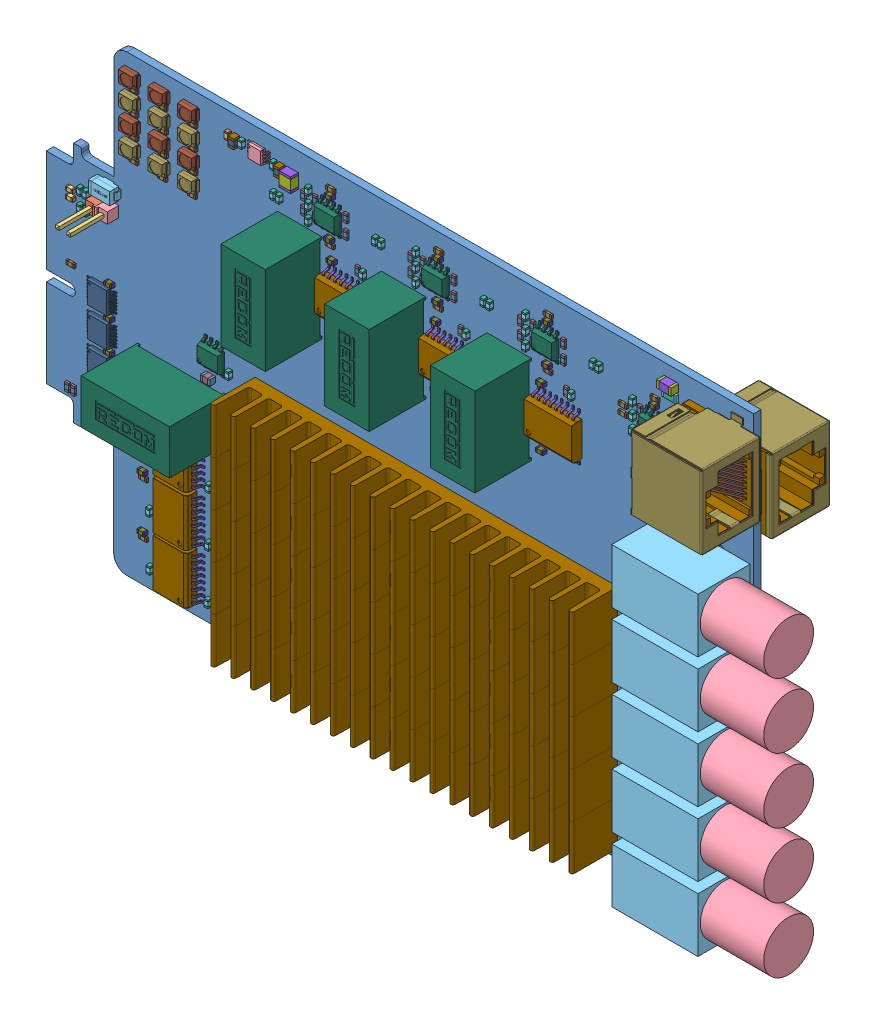
SolidWorks assembly 1166V10, configuration Standard. Lengths in mm. (continued)
Components (placement in the parent): (continued)
- 1166V10.step-1: 1166V10.step [Standard] at origin size (170.01 100 28.53) (continued)
  - C233.step-1: C233.step [Standard] at origin size (0.82 1.6 0.9) (continued)
    - 6549602528.step-1: 6549602528.step [Standard] at (39.6 30.325 -2.522) size (0.82 0.35 0.9) (continued)
      - Extruded-0.step-1: Extruded-0.step [Standard] at origin size (0.82 0.35 0.9)
    - 6549602528.step-2: 6549602528.step [Standard] at (39.6 31.575 -2.522) size (0.82 0.35 0.9)
      - Extruded-0.step-1: Extruded-0.step [Standard] at origin size (0.82 0.35 0.9)
    - 6547668352.step-1: 6547668352.step [Standard] at (39.6 30.95 -2.522) size (0.82 0.9 0.9)
      - Extruded.step-1: Extruded.step [Standard] at origin size (0.82 0.9 0.9)
  - C232.step-1: C232.step [Standard] at origin size (0.82 1.6 0.9)
    - 6547668352.step-1: 6547668352.step [Standard] at (106.1 91.15 0) size (0.82 0.9 0.9)
      - Extruded.step-1: Extruded.step [Standard] at origin size (0.82 0.9 0.9)
    - 6549602528.step-1: 6549602528.step [Standard] at (106.1 91.775 0) size (0.82 0.35 0.9)
      - Extruded-0.step-1: Extruded-0.step [Standard] at origin size (0.82 0.35 0.9)
    - 6549602528.step-2: 6549602528.step [Standard] at (106.1 90.525 0) size (0.82 0.35 0.9)
      - Extruded-0.step-1: Extruded-0.step [Standard] at origin size (0.82 0.35 0.9)
  - C231.step-1: C231.step [Standard] at origin size (0.82 1.6 0.9)
    - 6547668352.step-1: 6547668352.step [Standard] at (106.1 94.05 0) size (0.82 0.9 0.9)
      - Extruded.step-1: Extruded.step [Standard] at origin size (0.82 0.9 0.9)
    - 6549602528.step-1: 6549602528.step [Standard] at (106.1 94.675 0) size (0.82 0.35 0.9)
      - Extruded-0.step-1: Extruded-0.step [Standard] at origin size (0.82 0.35 0.9)
    - 6549602528.step-2: 6549602528.step [Standard] at (106.1 93.425 0) size (0.82 0.35 0.9)
      - Extruded-0.step-1: Extruded-0.step [Standard] at origin size (0.82 0.35 0.9)
  - R101.step-1: R101.step [Standard] at origin size (1.85 0.85 0.45)
    - 6547171712.step-1: 6547171712.step [Standard] at (4.95 53.6 0) size (0.45 0.85 0.45)
      - Extruded-5.step-1: Extruded-5.step [Standard] at origin size (0.45 0.85 0.45)
    - 6547171712.step-2: 6547171712.step [Standard] at (6.35 53.6 0) size (0.45 0.85 0.45)
      - Extruded-5.step-1: Extruded-5.step [Standard] at origin size (0.45 0.85 0.45)
    - 6547171152.step-1: 6547171152.step [Standard] at (5.65 53.6 0) size (0.95 0.85 0.45)
      - Extruded-6.step-1: Extruded-6.step [Standard] at origin size (0.95 0.85 0.45)
  - CF101.step-1: CF101.step [Standard] at origin size (1.6 0.82 0.9)
    - 6547664912.step-1: 6547664912.step [Standard] at (13.725 54.2 0) size (0.35 0.82 0.9)
      - Extruded-10.step-1: Extruded-10.step [Standard] at origin size (0.35 0.82 0.9)
    - 6547664912.step-2: 6547664912.step [Standard] at (14.975 54.2 0) size (0.35 0.82 0.9)
      - Extruded-10.step-1: Extruded-10.step [Standard] at origin size (0.35 0.82 0.9)
    - 6547664352.step-1: 6547664352.step [Standard] at (14.35 54.2 0) size (0.9 0.82 0.9)
      - Extruded-9.step-1: Extruded-9.step [Standard] at origin size (0.9 0.82 0.9)
  - PS202.step-1: PS202.step [Standard] at origin size (19.5 9.8 16.6)
    - RxxPxx_X2_R.step-1: RxxPxx_X2_R.step [Standard] at (29.9099 40.6999 0.51) x (1 0 0) z (0 -1 0) size (0.5 4.6 0.25)
    - RxxPxx_X2_R-24.step-1: RxxPxx_X2_R-24.step [Standard] at (29.9099 40.6999 0.51) x (1 0 0) z (0 -1 0) size (0.5 4.6 0.25)
    - RxxPxx_X2_R-25.step-1: RxxPxx_X2_R-25.step [Standard] at (29.9099 40.6999 0.51) x (1 0 0) z (0 -1 0) size (19.5 12.5 9.8)
    - RxxPxx_X2_R-26.step-1: RxxPxx_X2_R-26.step [Standard] at (29.9099 40.6999 0.51) x (1 0 0) z (0 -1 0) size (18.5 11.5 8.9)
    - RxxPxx_X2_R-27.step-1: RxxPxx_X2_R-27.step [Standard] at (29.9099 40.6999 0.51) x (1 0 0) z (0 -1 0) size (0.5 4.6 0.25)
    - RxxPxx_X2_R-28.step-1: RxxPxx_X2_R-28.step [Standard] at (29.9099 40.6999 0.51) x (1 0 0) z (0 -1 0) size (0.5 4.6 0.25)
  - PS401.step-1: PS401.step [Standard] at origin size (9.8 19.5 16.6)
    - RxxPxx_X2_R.step-1: RxxPxx_X2_R.step [Standard] at (55.8999 76.45 0.51) x (0 -1 0) z (-1 0 0) size (0.5 4.6 0.25)
    - RxxPxx_X2_R-24.step-1: RxxPxx_X2_R-24.step [Standard] at (55.8999 76.45 0.51) x (0 -1 0) z (-1 0 0) size (0.5 4.6 0.25)
    - RxxPxx_X2_R-25.step-1: RxxPxx_X2_R-25.step [Standard] at (55.8999 76.45 0.51) x (0 -1 0) z (-1 0 0) size (19.5 12.5 9.8)
    - RxxPxx_X2_R-26.step-1: RxxPxx_X2_R-26.step [Standard] at (55.8999 76.45 0.51) x (0 -1 0) z (-1 0 0) size (18.5 11.5 8.9)
    - RxxPxx_X2_R-27.step-1: RxxPxx_X2_R-27.step [Standard] at (55.8999 76.45 0.51) x (0 -1 0) z (-1 0 0) size (0.5 4.6 0.25)
    - RxxPxx_X2_R-28.step-1: RxxPxx_X2_R-28.step [Standard] at (55.8999 76.45 0.51) x (0 -1 0) z (-1 0 0) size (0.5 4.6 0.25)
  - PS301.step-1: PS301.step [Standard] at origin size (9.8 19.5 16.6)
    - RxxPxx_X2_R.step-1: RxxPxx_X2_R.step [Standard] at (78.7999 76.45 0.51) x (0 -1 0) z (-1 0 0) size (0.5 4.6 0.25)
    - RxxPxx_X2_R-24.step-1: RxxPxx_X2_R-24.step [Standard] at (78.7999 76.45 0.51) x (0 -1 0) z (-1 0 0) size (0.5 4.6 0.25)
    - RxxPxx_X2_R-25.step-1: RxxPxx_X2_R-25.step [Standard] at (78.7999 76.45 0.51) x (0 -1 0) z (-1 0 0) size (19.5 12.5 9.8)
    - RxxPxx_X2_R-26.step-1: RxxPxx_X2_R-26.step [Standard] at (78.7999 76.45 0.51) x (0 -1 0) z (-1 0 0) size (18.5 11.5 8.9)
    - RxxPxx_X2_R-27.step-1: RxxPxx_X2_R-27.step [Standard] at (78.7999 76.45 0.51) x (0 -1 0) z (-1 0 0) size (0.5 4.6 0.25)
    - RxxPxx_X2_R-28.step-1: RxxPxx_X2_R-28.step [Standard] at (78.7999 76.45 0.51) x (0 -1 0) z (-1 0 0) size (0.5 4.6 0.25)
  - L402.step-1: L402.step [Standard] at origin size (1.8 2 1.8)
    - 6547443440.step-1: 6547443440.step [Standard] at (56.3 66.0999 -3.422) size (1.8 0.5 1.8)
      - Extruded-29.step-1: Extruded-29.step [Standard] at origin size (1.8 0.5 1.8)
    - 6547443440.step-2: 6547443440.step [Standard] at (56.3 64.6 -3.422) size (1.8 0.5 1.8)
      - Extruded-29.step-1: Extruded-29.step [Standard] at origin size (1.8 0.5 1.8)
    - 6547443040.step-1: 6547443040.step [Standard] at (56.3 65.3499 -3.422) size (1.8 1 1.8)
      - Extruded-30.step-1: Extruded-30.step [Standard] at origin size (1.8 1 1.8)
  - L401.step-1: L401.step [Standard] at origin size (1.8 2 1.8)
    - 6547443440.step-1: 6547443440.step [Standard] at (56.9 89.3999 -3.422) size (1.8 0.5 1.8)
      - Extruded-29.step-1: Extruded-29.step [Standard] at origin size (1.8 0.5 1.8)
    - 6547443440.step-2: 6547443440.step [Standard] at (56.9 87.9 -3.422) size (1.8 0.5 1.8)
      - Extruded-29.step-1: Extruded-29.step [Standard] at origin size (1.8 0.5 1.8)
    - 6547443040.step-1: 6547443040.step [Standard] at (56.8999 88.6499 -3.422) size (1.8 1 1.8)
      - Extruded-30.step-1: Extruded-30.step [Standard] at origin size (1.8 1 1.8)
  - L302.step-1: L302.step [Standard] at origin size (1.8 2 1.8)
    - 6547443440.step-1: 6547443440.step [Standard] at (79.2 66.0999 -3.422) size (1.8 0.5 1.8)
      - Extruded-29.step-1: Extruded-29.step [Standard] at origin size (1.8 0.5 1.8)
    - 6547443440.step-2: 6547443440.step [Standard] at (79.2 64.6 -3.422) size (1.8 0.5 1.8)
      - Extruded-29.step-1: Extruded-29.step [Standard] at origin size (1.8 0.5 1.8)
    - 6547443040.step-1: 6547443040.step [Standard] at (79.1999 65.3499 -3.422) size (1.8 1 1.8)
      - Extruded-30.step-1: Extruded-30.step [Standard] at origin size (1.8 1 1.8)
  - L301.step-1: L301.step [Standard] at origin size (1.8 2 1.8)
    - 6547443440.step-1: 6547443440.step [Standard] at (79.4 89.3999 -3.422) size (1.8 0.5 1.8)
      - Extruded-29.step-1: Extruded-29.step [Standard] at origin size (1.8 0.5 1.8)
    - 6547443440.step-2: 6547443440.step [Standard] at (79.4 87.9 -3.422) size (1.8 0.5 1.8)
      - Extruded-29.step-1: Extruded-29.step [Standard] at origin size (1.8 0.5 1.8)
    - 6547443040.step-1: 6547443040.step [Standard] at (79.3999 88.6499 -3.422) size (1.8 1 1.8)
      - Extruded-30.step-1: Extruded-30.step [Standard] at origin size (1.8 1 1.8)
  - J401.step-1: J401.step [Standard] at origin size (33 12 11.5)
    - 6544611248.step-1: 6544611248.step [Standard] at (146.5 8.5 0.8) size (19 12 11.5)
      - Extruded-21.step-1: Extruded-21.step [Standard] at origin size (19 12 11.5)
    - 6544611488.step-1: 6544611488.step [Standard] at (170 8.5434 6.3) x (0 -1 0) z (-1 0 0) size (11 11 14)
      - Cylinder.step-1: Cylinder.step [Standard] at origin size (11 11 14)
  - J301.step-1: J301.step [Standard] at origin size (33 12 11.5)
    - 6544611248.step-1: 6544611248.step [Standard] at (146.5 22.8 0.8) size (19 12 11.5)
      - Extruded-21.step-1: Extruded-21.step [Standard] at origin size (19 12 11.5)
    - 6544611488.step-1: 6544611488.step [Standard] at (170 22.8434 6.3) x (0 -1 0) z (-1 0 0) size (11 11 14)
      - Cylinder.step-1: Cylinder.step [Standard] at origin size (11 11 14)
  - CF405.step-1: CF405.step [Standard] at origin size (0.82 1.6 0.9)
    - 6547668352.step-1: 6547668352.step [Standard] at (23.2 26.35 0) size (0.82 0.9 0.9)
      - Extruded.step-1: Extruded.step [Standard] at origin size (0.82 0.9 0.9)
    - 6549602528.step-1: 6549602528.step [Standard] at (23.2 26.975 0) size (0.82 0.35 0.9)
      - Extruded-0.step-1: Extruded-0.step [Standard] at origin size (0.82 0.35 0.9)
    - 6549602528.step-2: 6549602528.step [Standard] at (23.2 25.725 0) size (0.82 0.35 0.9)
      - Extruded-0.step-1: Extruded-0.step [Standard] at origin size (0.82 0.35 0.9)
  - CF402.step-1: CF402.step [Standard] at origin size (2.1 1.25 1.3)
    - 6545928368.step-1: 6545928368.step [Standard] at (58.7 64.6 -2.922) size (0.5 1.25 1.3)
      - Extruded-16.step-1: Extruded-16.step [Standard] at origin size (0.5 1.25 1.3)
    - 6545928368.step-2: 6545928368.step [Standard] at (60.3 64.6 -2.922) size (0.5 1.25 1.3)
      - Extruded-16.step-1: Extruded-16.step [Standard] at origin size (0.5 1.25 1.3)
    - 6545927808.step-1: 6545927808.step [Standard] at (59.5 64.6 -2.922) size (1.1 1.25 1.3)
      - Extruded-15.step-1: Extruded-15.step [Standard] at origin size (1.1 1.25 1.3)
  - CF401.step-1: CF401.step [Standard] at origin size (2.1 1.25 1.3)
    - 6545928368.step-1: 6545928368.step [Standard] at (58.7 66.4 -2.922) size (0.5 1.25 1.3)
      - Extruded-16.step-1: Extruded-16.step [Standard] at origin size (0.5 1.25 1.3)
    - 6545928368.step-2: 6545928368.step [Standard] at (60.3 66.4 -2.922) size (0.5 1.25 1.3)
      - Extruded-16.step-1: Extruded-16.step [Standard] at origin size (0.5 1.25 1.3)
    - 6545927808.step-1: 6545927808.step [Standard] at (59.5 66.4 -2.922) size (1.1 1.25 1.3)
      - Extruded-15.step-1: Extruded-15.step [Standard] at origin size (1.1 1.25 1.3)
  - CF403.step-1: CF403.step [Standard] at origin size (1.6 0.82 0.9)
    - 6547664352.step-1: 6547664352.step [Standard] at (63.35 83.1 0) size (0.9 0.82 0.9)
      - Extruded-9.step-1: Extruded-9.step [Standard] at origin size (0.9 0.82 0.9)
    - 6547664912.step-1: 6547664912.step [Standard] at (63.975 83.1 0) size (0.35 0.82 0.9)
      - Extruded-10.step-1: Extruded-10.step [Standard] at origin size (0.35 0.82 0.9)
    - 6547664912.step-2: 6547664912.step [Standard] at (62.725 83.1 0) size (0.35 0.82 0.9)
      - Extruded-10.step-1: Extruded-10.step [Standard] at origin size (0.35 0.82 0.9)
  - CF305.step-1: CF305.step [Standard] at origin size (0.82 1.6 0.9)
    - 6547668352.step-1: 6547668352.step [Standard] at (23.2 15.25 0) size (0.82 0.9 0.9)
      - Extruded.step-1: Extruded.step [Standard] at origin size (0.82 0.9 0.9)
    - 6549602528.step-1: 6549602528.step [Standard] at (23.2 15.875 0) size (0.82 0.35 0.9)
      - Extruded-0.step-1: Extruded-0.step [Standard] at origin size (0.82 0.35 0.9)
    - 6549602528.step-2: 6549602528.step [Standard] at (23.2 14.625 0) size (0.82 0.35 0.9)
      - Extruded-0.step-1: Extruded-0.step [Standard] at origin size (0.82 0.35 0.9)
  - CF302.step-1: CF302.step [Standard] at origin size (2.1 1.25 1.3)
    - 6545928368.step-1: 6545928368.step [Standard] at (81.6 64.6 -2.922) size (0.5 1.25 1.3)
      - Extruded-16.step-1: Extruded-16.step [Standard] at origin size (0.5 1.25 1.3)
    - 6545928368.step-2: 6545928368.step [Standard] at (83.2 64.6 -2.922) size (0.5 1.25 1.3)
      - Extruded-16.step-1: Extruded-16.step [Standard] at origin size (0.5 1.25 1.3)
    - 6545927808.step-1: 6545927808.step [Standard] at (82.4 64.6 -2.922) size (1.1 1.25 1.3)
      - Extruded-15.step-1: Extruded-15.step [Standard] at origin size (1.1 1.25 1.3)
  - CF301.step-1: CF301.step [Standard] at origin size (2.1 1.25 1.3)
    - 6545928368.step-1: 6545928368.step [Standard] at (81.6 66.4 -2.922) size (0.5 1.25 1.3)
      - Extruded-16.step-1: Extruded-16.step [Standard] at origin size (0.5 1.25 1.3)
    - 6545928368.step-2: 6545928368.step [Standard] at (83.2 66.4 -2.922) size (0.5 1.25 1.3)
      - Extruded-16.step-1: Extruded-16.step [Standard] at origin size (0.5 1.25 1.3)
    - 6545927808.step-1: 6545927808.step [Standard] at (82.4 66.4 -2.922) size (1.1 1.25 1.3)
      - Extruded-15.step-1: Extruded-15.step [Standard] at origin size (1.1 1.25 1.3)
  - CF303.step-1: CF303.step [Standard] at origin size (1.6 0.82 0.9)
    - 6547664352.step-1: 6547664352.step [Standard] at (86.25 83 0) size (0.9 0.82 0.9)
      - Extruded-9.step-1: Extruded-9.step [Standard] at origin size (0.9 0.82 0.9)
    - 6547664912.step-1: 6547664912.step [Standard] at (86.875 83 0) size (0.35 0.82 0.9)
      - Extruded-10.step-1: Extruded-10.step [Standard] at origin size (0.35 0.82 0.9)
    - 6547664912.step-2: 6547664912.step [Standard] at (85.625 83 0) size (0.35 0.82 0.9)
      - Extruded-10.step-1: Extruded-10.step [Standard] at origin size (0.35 0.82 0.9)
  - C410.step-1: C410.step [Standard] at origin size (1.6 0.82 0.9)
    - 6547664912.step-1: 6547664912.step [Standard] at (58.625 63.1 -2.522) size (0.35 0.82 0.9)
      - Extruded-10.step-1: Extruded-10.step [Standard] at origin size (0.35 0.82 0.9)
    - 6547664912.step-2: 6547664912.step [Standard] at (59.875 63.1 -2.522) size (0.35 0.82 0.9)
      - Extruded-10.step-1: Extruded-10.step [Standard] at origin size (0.35 0.82 0.9)
    - 6547664352.step-1: 6547664352.step [Standard] at (59.25 63.1 -2.522) size (0.9 0.82 0.9)
      - Extruded-9.step-1: Extruded-9.step [Standard] at origin size (0.9 0.82 0.9)
  - C409.step-1: C409.step [Standard] at origin size (3.2 1.6 1.7)
    - 6547445040.step-1: 6547445040.step [Standard] at (60.55 87.7 -3.322) size (2.2 1.6 1.7)
      - Extruded-23.step-1: Extruded-23.step [Standard] at origin size (2.2 1.6 1.7)
    - 6547444720.step-1: 6547444720.step [Standard] at (59.2 87.7 -3.322) size (0.5 1.6 1.7)
      - Extruded-22.step-1: Extruded-22.step [Standard] at origin size (0.5 1.6 1.7)
    - 6547444720.step-2: 6547444720.step [Standard] at (61.9 87.7 -3.322) size (0.5 1.6 1.7)
      - Extruded-22.step-1: Extruded-22.step [Standard] at origin size (0.5 1.6 1.7)
  - C408.step-1: C408.step [Standard] at origin size (3.2 1.6 1.7)
    - 6547445040.step-1: 6547445040.step [Standard] at (60.55 89.8 -3.322) size (2.2 1.6 1.7)
      - Extruded-23.step-1: Extruded-23.step [Standard] at origin size (2.2 1.6 1.7)
    - 6547444720.step-1: 6547444720.step [Standard] at (59.2 89.8 -3.322) size (0.5 1.6 1.7)
      - Extruded-22.step-1: Extruded-22.step [Standard] at origin size (0.5 1.6 1.7)
    - 6547444720.step-2: 6547444720.step [Standard] at (61.9 89.8 -3.322) size (0.5 1.6 1.7)
      - Extruded-22.step-1: Extruded-22.step [Standard] at origin size (0.5 1.6 1.7)
  - C407.step-1: C407.step [Standard] at origin size (5.7 5 2.5)
    - 6545673168.step-1: 6545673168.step [Standard] at (66.25 49.3 -4.122) size (4.4 5 2.5)
      - Extruded-31.step-1: Extruded-31.step [Standard] at origin size (4.4 5 2.5)
    - 6545673728.step-1: 6545673728.step [Standard] at (68.775 49.3 -4.122) size (0.65 5 2.5)
      - Extruded-32.step-1: Extruded-32.step [Standard] at origin size (0.65 5 2.5)
    - 6545673728.step-2: 6545673728.step [Standard] at (63.725 49.3 -4.122) size (0.65 5 2.5)
      - Extruded-32.step-1: Extruded-32.step [Standard] at origin size (0.65 5 2.5)
  - C406.step-1: C406.step [Standard] at origin size (5.7 5 2.5)
    - 6545673728.step-1: 6545673728.step [Standard] at (56.375 43.2 -4.122) size (0.65 5 2.5)
      - Extruded-32.step-1: Extruded-32.step [Standard] at origin size (0.65 5 2.5)
    - 6545673728.step-2: 6545673728.step [Standard] at (51.325 43.2 -4.122) size (0.65 5 2.5)
      - Extruded-32.step-1: Extruded-32.step [Standard] at origin size (0.65 5 2.5)
    - 6545673168.step-1: 6545673168.step [Standard] at (53.85 43.2 -4.122) size (4.4 5 2.5)
      - Extruded-31.step-1: Extruded-31.step [Standard] at origin size (4.4 5 2.5)
  - C405.step-1: C405.step [Standard] at origin size (5.7 5 2.5)
    - 6545673728.step-1: 6545673728.step [Standard] at (56.375 49.3 -4.122) size (0.65 5 2.5)
      - Extruded-32.step-1: Extruded-32.step [Standard] at origin size (0.65 5 2.5)
    - 6545673728.step-2: 6545673728.step [Standard] at (51.325 49.3 -4.122) size (0.65 5 2.5)
      - Extruded-32.step-1: Extruded-32.step [Standard] at origin size (0.65 5 2.5)
    - 6545673168.step-1: 6545673168.step [Standard] at (53.85 49.3 -4.122) size (4.4 5 2.5)
      - Extruded-31.step-1: Extruded-31.step [Standard] at origin size (4.4 5 2.5)
  - C404.step-1: C404.step [Standard] at origin size (5.7 5 2.5)
    - 6545673728.step-1: 6545673728.step [Standard] at (63.725 43.2 -4.122) size (0.65 5 2.5)
      - Extruded-32.step-1: Extruded-32.step [Standard] at origin size (0.65 5 2.5)
    - 6545673728.step-2: 6545673728.step [Standard] at (68.775 43.2 -4.122) size (0.65 5 2.5)
      - Extruded-32.step-1: Extruded-32.step [Standard] at origin size (0.65 5 2.5)
    - 6545673168.step-1: 6545673168.step [Standard] at (66.25 43.2 -4.122) size (4.4 5 2.5)
      - Extruded-31.step-1: Extruded-31.step [Standard] at origin size (4.4 5 2.5)
  - C310.step-1: C310.step [Standard] at origin size (1.6 0.82 0.9)
    - 6547664912.step-1: 6547664912.step [Standard] at (82.025 63 -2.522) size (0.35 0.82 0.9)
      - Extruded-10.step-1: Extruded-10.step [Standard] at origin size (0.35 0.82 0.9)
    - 6547664912.step-2: 6547664912.step [Standard] at (83.275 63 -2.522) size (0.35 0.82 0.9)
      - Extruded-10.step-1: Extruded-10.step [Standard] at origin size (0.35 0.82 0.9)
    - 6547664352.step-1: 6547664352.step [Standard] at (82.65 63 -2.522) size (0.9 0.82 0.9)
      - Extruded-9.step-1: Extruded-9.step [Standard] at origin size (0.9 0.82 0.9)
  - C309.step-1: C309.step [Standard] at origin size (3.2 1.6 1.7)
    - 6547445040.step-1: 6547445040.step [Standard] at (83.05 87.6 -3.322) size (2.2 1.6 1.7)
      - Extruded-23.step-1: Extruded-23.step [Standard] at origin size (2.2 1.6 1.7)
    - 6547444720.step-1: 6547444720.step [Standard] at (81.7 87.6 -3.322) size (0.5 1.6 1.7)
      - Extruded-22.step-1: Extruded-22.step [Standard] at origin size (0.5 1.6 1.7)
    - 6547444720.step-2: 6547444720.step [Standard] at (84.4 87.6 -3.322) size (0.5 1.6 1.7)
      - Extruded-22.step-1: Extruded-22.step [Standard] at origin size (0.5 1.6 1.7)
  - C308.step-1: C308.step [Standard] at origin size (3.2 1.6 1.7)
    - 6547445040.step-1: 6547445040.step [Standard] at (83.05 89.7 -3.322) size (2.2 1.6 1.7)
      - Extruded-23.step-1: Extruded-23.step [Standard] at origin size (2.2 1.6 1.7)
    - 6547444720.step-1: 6547444720.step [Standard] at (81.7 89.7 -3.322) size (0.5 1.6 1.7)
      - Extruded-22.step-1: Extruded-22.step [Standard] at origin size (0.5 1.6 1.7)
    - 6547444720.step-2: 6547444720.step [Standard] at (84.4 89.7 -3.322) size (0.5 1.6 1.7)
      - Extruded-22.step-1: Extruded-22.step [Standard] at origin size (0.5 1.6 1.7)
  - C307.step-1: C307.step [Standard] at origin size (5.7 5 2.5)
    - 6545673168.step-1: 6545673168.step [Standard] at (93.15 49.3 -4.122) size (4.4 5 2.5)
      - Extruded-31.step-1: Extruded-31.step [Standard] at origin size (4.4 5 2.5)
    - 6545673728.step-1: 6545673728.step [Standard] at (95.675 49.3 -4.122) size (0.65 5 2.5)
      - Extruded-32.step-1: Extruded-32.step [Standard] at origin size (0.65 5 2.5)
    - 6545673728.step-2: 6545673728.step [Standard] at (90.625 49.3 -4.122) size (0.65 5 2.5)
      - Extruded-32.step-1: Extruded-32.step [Standard] at origin size (0.65 5 2.5)
  - C306.step-1: C306.step [Standard] at origin size (5.7 5 2.5)
    - 6545673728.step-1: 6545673728.step [Standard] at (83.375 49.3 -4.122) size (0.65 5 2.5)
      - Extruded-32.step-1: Extruded-32.step [Standard] at origin size (0.65 5 2.5)
    - 6545673728.step-2: 6545673728.step [Standard] at (78.325 49.3 -4.122) size (0.65 5 2.5)
      - Extruded-32.step-1: Extruded-32.step [Standard] at origin size (0.65 5 2.5)
    - 6545673168.step-1: 6545673168.step [Standard] at (80.85 49.3 -4.122) size (4.4 5 2.5)
      - Extruded-31.step-1: Extruded-31.step [Standard] at origin size (4.4 5 2.5)
  - C305.step-1: C305.step [Standard] at origin size (5.7 5 2.5)
    - 6545673728.step-1: 6545673728.step [Standard] at (83.375 43.2 -4.122) size (0.65 5 2.5)
      - Extruded-32.step-1: Extruded-32.step [Standard] at origin size (0.65 5 2.5)
    - 6545673728.step-2: 6545673728.step [Standard] at (78.325 43.2 -4.122) size (0.65 5 2.5)
      - Extruded-32.step-1: Extruded-32.step [Standard] at origin size (0.65 5 2.5)
    - 6545673168.step-1: 6545673168.step [Standard] at (80.85 43.2 -4.122) size (4.4 5 2.5)
      - Extruded-31.step-1: Extruded-31.step [Standard] at origin size (4.4 5 2.5)
  - C304.step-1: C304.step [Standard] at origin size (5.7 5 2.5)
    - 6545673728.step-1: 6545673728.step [Standard] at (90.625 43.2 -4.122) size (0.65 5 2.5)
      - Extruded-32.step-1: Extruded-32.step [Standard] at origin size (0.65 5 2.5)
    - 6545673728.step-2: 6545673728.step [Standard] at (95.675 43.2 -4.122) size (0.65 5 2.5)
      - Extruded-32.step-1: Extruded-32.step [Standard] at origin size (0.65 5 2.5)
    - 6545673168.step-1: 6545673168.step [Standard] at (93.15 43.2 -4.122) size (4.4 5 2.5)
      - Extruded-31.step-1: Extruded-31.step [Standard] at origin size (4.4 5 2.5)
  - L101.step-1: L101.step [Standard] at origin size (1.6 0.8 0.8)
    - WE-CBF_0603_CBF.step-1: WE-CBF_0603_CBF.step [Standard] at (5.7637 68.0001 0.4) x (0 1 0) z (0 0 1) size (0.8 1.6 0.8)
      - L_tende.step-1: L_tende.step [Standard] at (0 -0.5 0) size (0.8 0.3 0.8)
      - L_tende.step-2: L_tende.step [Standard] at (0 0.5 0) x (-1 0 0) z (0 0 1) size (0.8 0.3 0.8)
      - base.step-1: base.step [Standard] at origin size (0.8 1 0.8)
  - C102.step-1: C102.step [Standard] at origin size (0.82 1.6 0.9)
    - 6547668352.step-1: 6547668352.step [Standard] at (9.2 68.85 0) size (0.82 0.9 0.9)
      - Extruded.step-1: Extruded.step [Standard] at origin size (0.82 0.9 0.9)
    - 6549602528.step-1: 6549602528.step [Standard] at (9.2 68.225 0) size (0.82 0.35 0.9)
      - Extruded-0.step-1: Extruded-0.step [Standard] at origin size (0.82 0.35 0.9)
    - 6549602528.step-2: 6549602528.step [Standard] at (9.2 69.475 0) size (0.82 0.35 0.9)
      - Extruded-0.step-1: Extruded-0.step [Standard] at origin size (0.82 0.35 0.9)
  - C101.step-1: C101.step [Standard] at origin size (0.82 1.6 0.9)
    - 6547668352.step-1: 6547668352.step [Standard] at (7.9 68.85 0) size (0.82 0.9 0.9)
      - Extruded.step-1: Extruded.step [Standard] at origin size (0.82 0.9 0.9)
    - 6549602528.step-1: 6549602528.step [Standard] at (7.9 68.225 0) size (0.82 0.35 0.9)
      - Extruded-0.step-1: Extruded-0.step [Standard] at origin size (0.82 0.35 0.9)
    - 6549602528.step-2: 6549602528.step [Standard] at (7.9 69.475 0) size (0.82 0.35 0.9)
      - Extruded-0.step-1: Extruded-0.step [Standard] at origin size (0.82 0.35 0.9)
  - J201.step-1: J201.step [Standard] at origin size (33 12 11.5)
    - 6544611248.step-1: 6544611248.step [Standard] at (146.5 37.1 0.8) size (19 12 11.5)
      - Extruded-21.step-1: Extruded-21.step [Standard] at origin size (19 12 11.5)
    - 6544611488.step-1: 6544611488.step [Standard] at (170 37.1433 6.3) x (0 -1 0) z (-1 0 0) size (11 11 14)
      - Cylinder.step-1: Cylinder.step [Standard] at origin size (11 11 14)
  - RX101.step-1: RX101.step [Standard] at origin size (3.2 1.6 0.55)
    - 6543827536.step-1: 6543827536.step [Standard] at (139.225 94.6 0) size (0.45 1.6 0.55)
      - Extruded-33.step-1: Extruded-33.step [Standard] at origin size (0.45 1.6 0.55)
    - 6543827536.step-2: 6543827536.step [Standard] at (136.475 94.6 0) size (0.45 1.6 0.55)
      - Extruded-33.step-1: Extruded-33.step [Standard] at origin size (0.45 1.6 0.55)
    - 6543826896.step-1: 6543826896.step [Standard] at (137.85 94.6 0) size (2.3 1.6 0.55)
      - Extruded-34.step-1: Extruded-34.step [Standard] at origin size (2.3 1.6 0.55)
  - R103.step-1: R103.step [Standard] at origin size (0.85 1.85 0.45)
    - 6549605488.step-1: 6549605488.step [Standard] at (4.9 29.75 0) size (0.85 0.95 0.45)
      - Extruded-8.step-1: Extruded-8.step [Standard] at origin size (0.85 0.95 0.45)
    - 6549605008.step-1: 6549605008.step [Standard] at (4.9 30.45 0) size (0.85 0.45 0.45)
      - Extruded-7.step-1: Extruded-7.step [Standard] at origin size (0.85 0.45 0.45)
    - 6549605008.step-2: 6549605008.step [Standard] at (4.9 29.05 0) size (0.85 0.45 0.45)
      - Extruded-7.step-1: Extruded-7.step [Standard] at origin size (0.85 0.45 0.45)
  - R102.step-1: R102.step [Standard] at origin size (0.85 1.85 0.45)
    - 6549605488.step-1: 6549605488.step [Standard] at (6.2 29.75 0) size (0.85 0.95 0.45)
      - Extruded-8.step-1: Extruded-8.step [Standard] at origin size (0.85 0.95 0.45)
    - 6549605008.step-1: 6549605008.step [Standard] at (6.2 29.05 0) size (0.85 0.45 0.45)
      - Extruded-7.step-1: Extruded-7.step [Standard] at origin size (0.85 0.45 0.45)
    - 6549605008.step-2: 6549605008.step [Standard] at (6.2 30.45 0) size (0.85 0.45 0.45)
      - Extruded-7.step-1: Extruded-7.step [Standard] at origin size (0.85 0.45 0.45)
  - PS201.step-1: PS201.step [Standard] at origin size (9.8 19.5 16.6)
    - RxxPxx_X2_R.step-1: RxxPxx_X2_R.step [Standard] at (102.0999 76.3501 0.51) x (0 -1 0) z (-1 0 0) size (0.5 4.6 0.25)
    - RxxPxx_X2_R-24.step-1: RxxPxx_X2_R-24.step [Standard] at (102.0999 76.3501 0.51) x (0 -1 0) z (-1 0 0) size (0.5 4.6 0.25)
    - RxxPxx_X2_R-25.step-1: RxxPxx_X2_R-25.step [Standard] at (102.0999 76.3501 0.51) x (0 -1 0) z (-1 0 0) size (19.5 12.5 9.8)
    - RxxPxx_X2_R-26.step-1: RxxPxx_X2_R-26.step [Standard] at (102.0999 76.3501 0.51) x (0 -1 0) z (-1 0 0) size (18.5 11.5 8.9)
    - RxxPxx_X2_R-27.step-1: RxxPxx_X2_R-27.step [Standard] at (102.0999 76.3501 0.51) x (0 -1 0) z (-1 0 0) size (0.5 4.6 0.25)
    - RxxPxx_X2_R-28.step-1: RxxPxx_X2_R-28.step [Standard] at (102.0999 76.3501 0.51) x (0 -1 0) z (-1 0 0) size (0.5 4.6 0.25)
  - L205.step-1: L205.step [Standard] at origin size (2 1.8 1.8)
    - 6547446480.step-1: 6547446480.step [Standard] at (41 45.2 -3.422) size (0.5 1.8 1.8)
      - Extruded-35.step-1: Extruded-35.step [Standard] at origin size (0.5 1.8 1.8)
    - 6547446480.step-2: 6547446480.step [Standard] at (42.5 45.2 -3.422) size (0.5 1.8 1.8)
      - Extruded-35.step-1: Extruded-35.step [Standard] at origin size (0.5 1.8 1.8)
    - 6547446080.step-1: 6547446080.step [Standard] at (41.7501 45.1999 -3.422) size (1 1.8 1.8)
      - Extruded-36.step-1: Extruded-36.step [Standard] at origin size (1 1.8 1.8)
  - L204.step-1: L204.step [Standard] at origin size (1.8 2 1.8)
    - 6547443440.step-1: 6547443440.step [Standard] at (19.2 48.5 -3.422) size (1.8 0.5 1.8)
      - Extruded-29.step-1: Extruded-29.step [Standard] at origin size (1.8 0.5 1.8)
    - 6547443440.step-2: 6547443440.step [Standard] at (19.2 47 -3.422) size (1.8 0.5 1.8)
      - Extruded-29.step-1: Extruded-29.step [Standard] at origin size (1.8 0.5 1.8)
    - 6547443040.step-1: 6547443040.step [Standard] at (19.1999 47.7499 -3.422) size (1.8 1 1.8)
      - Extruded-30.step-1: Extruded-30.step [Standard] at origin size (1.8 1 1.8)
  - L202.step-1: L202.step [Standard] at origin size (1.8 2 1.8)
    - 6547443440.step-1: 6547443440.step [Standard] at (102.5 66.0999 -3.422) size (1.8 0.5 1.8)
      - Extruded-29.step-1: Extruded-29.step [Standard] at origin size (1.8 0.5 1.8)
    - 6547443440.step-2: 6547443440.step [Standard] at (102.5 64.6 -3.422) size (1.8 0.5 1.8)
      - Extruded-29.step-1: Extruded-29.step [Standard] at origin size (1.8 0.5 1.8)
    - 6547443040.step-1: 6547443040.step [Standard] at (102.5 65.3499 -3.422) size (1.8 1 1.8)
      - Extruded-30.step-1: Extruded-30.step [Standard] at origin size (1.8 1 1.8)
  - L201.step-1: L201.step [Standard] at origin size (1.8 2 1.8)
    - 6547443440.step-1: 6547443440.step [Standard] at (103.5 89.5 -3.422) size (1.8 0.5 1.8)
      - Extruded-29.step-1: Extruded-29.step [Standard] at origin size (1.8 0.5 1.8)
    - 6547443440.step-2: 6547443440.step [Standard] at (103.5 88 -3.422) size (1.8 0.5 1.8)
      - Extruded-29.step-1: Extruded-29.step [Standard] at origin size (1.8 0.5 1.8)
    - 6547443040.step-1: 6547443040.step [Standard] at (103.5 88.7499 -3.422) size (1.8 1 1.8)
      - Extruded-30.step-1: Extruded-30.step [Standard] at origin size (1.8 1 1.8)
  - L102.step-1: L102.step [Standard] at origin size (1.6 0.8 0.8)
    - WE-CBF_0603_CBF.step-1: WE-CBF_0603_CBF.step [Standard] at (5.7637 66.4001 0.4) x (0 1 0) z (0 0 1) size (0.8 1.6 0.8)
      - L_tende.step-1: L_tende.step [Standard] at (0 -0.5 0) size (0.8 0.3 0.8)
      - L_tende.step-2: L_tende.step [Standard] at (0 0.5 0) x (-1 0 0) z (0 0 1) size (0.8 0.3 0.8)
      - base.step-1: base.step [Standard] at origin size (0.8 1 0.8)
  - IC204.step-1: IC204.step [Standard] at origin size (10.6 10.5 2.6)
    - SOIC-16-300.step-1: SOIC-16-300.step [Standard] at (29.6999 7.8491 1.4) x (0 -1 0) z (-1 0 0) size (10.5 2.6 10.6)
      - User_Library-SOIC-16-300_pin_SOIC_SO-300_1.step-1: User_Library-SOIC-16-300_pin_SOIC_SO-300_1.step [Standard] at (0.635 0 -3.8) x (-1 0 0) z (0 0 -1) size (0.4 1.55 1.5)
      - User_Library-SOIC-16-300_pin_SOIC_SO-300_1.step-2: User_Library-SOIC-16-300_pin_SOIC_SO-300_1.step [Standard] at (1.905 0 -3.8) x (-1 0 0) z (0 0 -1) size (0.4 1.55 1.5)
      - User_Library-SOIC-16-300_pin_SOIC_SO-300_1.step-3: User_Library-SOIC-16-300_pin_SOIC_SO-300_1.step [Standard] at (4.445 0 -3.8) x (-1 0 0) z (0 0 -1) size (0.4 1.55 1.5)
      - User_Library-SOIC-16-300_SOIC_300_SOIC_10.5X7.6_1.step-1: User_Library-SOIC-16-300_SOIC_300_SOIC_10.5X7.6_1.step [Standard] at origin size (10.5 2.35 7.6)
      - User_Library-SOIC-16-300_pin_SOIC_SO-300_1.step-4: User_Library-SOIC-16-300_pin_SOIC_SO-300_1.step [Standard] at (-3.175 0 -3.8) x (-1 0 0) z (0 0 -1) size (0.4 1.55 1.5)
      - User_Library-SOIC-16-300_pin_SOIC_SO-300_1.step-5: User_Library-SOIC-16-300_pin_SOIC_SO-300_1.step [Standard] at (-3.175 0 3.8) size (0.4 1.55 1.5)
      - User_Library-SOIC-16-300_pin_SOIC_SO-300_1.step-6: User_Library-SOIC-16-300_pin_SOIC_SO-300_1.step [Standard] at (1.905 0 3.8) size (0.4 1.55 1.5)
      - User_Library-SOIC-16-300_pin_SOIC_SO-300_1.step-7: User_Library-SOIC-16-300_pin_SOIC_SO-300_1.step [Standard] at (-1.905 0 3.8) size (0.4 1.55 1.5)
      - User_Library-SOIC-16-300_pin_SOIC_SO-300_1.step-8: User_Library-SOIC-16-300_pin_SOIC_SO-300_1.step [Standard] at (0.635 0 3.8) size (0.4 1.55 1.5)
      - User_Library-SOIC-16-300_pin_SOIC_SO-300_1.step-9: User_Library-SOIC-16-300_pin_SOIC_SO-300_1.step [Standard] at (3.175 0 3.8) size (0.4 1.55 1.5)
      - User_Library-SOIC-16-300_pin_SOIC_SO-300_1.step-10: User_Library-SOIC-16-300_pin_SOIC_SO-300_1.step [Standard] at (4.445 0 3.8) size (0.4 1.55 1.5)
      - User_Library-SOIC-16-300_pin_SOIC_SO-300_1.step-11: User_Library-SOIC-16-300_pin_SOIC_SO-300_1.step [Standard] at (-0.635 0 -3.8) x (-1 0 0) z (0 0 -1) size (0.4 1.55 1.5)
      - User_Library-SOIC-16-300_pin_SOIC_SO-300_1.step-12: User_Library-SOIC-16-300_pin_SOIC_SO-300_1.step [Standard] at (-4.445 0 3.8) size (0.4 1.55 1.5)
      - User_Library-SOIC-16-300_pin_SOIC_SO-300_1.step-13: User_Library-SOIC-16-300_pin_SOIC_SO-300_1.step [Standard] at (3.175 0 -3.8) x (-1 0 0) z (0 0 -1) size (0.4 1.55 1.5)
      - User_Library-SOIC-16-300_pin_SOIC_SO-300_1.step-14: User_Library-SOIC-16-300_pin_SOIC_SO-300_1.step [Standard] at (-0.635 0 3.8) size (0.4 1.55 1.5)
      - User_Library-SOIC-16-300_pin_SOIC_SO-300_1.step-15: User_Library-SOIC-16-300_pin_SOIC_SO-300_1.step [Standard] at (-4.445 0 -3.8) x (-1 0 0) z (0 0 -1) size (0.4 1.55 1.5)
      - User_Library-SOIC-16-300_pin_SOIC_SO-300_1.step-16: User_Library-SOIC-16-300_pin_SOIC_SO-300_1.step [Standard] at (-1.905 0 -3.8) x (-1 0 0) z (0 0 -1) size (0.4 1.55 1.5)
  - CX101.step-1: CX101.step [Standard] at origin size (3.2 1.6 1.7)
    - 6547444720.step-1: 6547444720.step [Standard] at (139.2 96.7 0) size (0.5 1.6 1.7)
      - Extruded-22.step-1: Extruded-22.step [Standard] at origin size (0.5 1.6 1.7)
    - 6547444720.step-2: 6547444720.step [Standard] at (136.5 96.7 0) size (0.5 1.6 1.7)
      - Extruded-22.step-1: Extruded-22.step [Standard] at origin size (0.5 1.6 1.7)
    - 6547445040.step-1: 6547445040.step [Standard] at (137.85 96.7 0) size (2.2 1.6 1.7)
      - Extruded-23.step-1: Extruded-23.step [Standard] at origin size (2.2 1.6 1.7)
  - CF206.step-1: CF206.step [Standard] at origin size (1.25 2.1 1.3)
    - 6549603568.step-1: 6549603568.step [Standard] at (42.56 42.9 -2.922) size (1.25 0.5 1.3)
      - Extruded-3.step-1: Extruded-3.step [Standard] at origin size (1.25 0.5 1.3)
    - 6549603568.step-2: 6549603568.step [Standard] at (42.56 41.3 -2.922) size (1.25 0.5 1.3)
      - Extruded-3.step-1: Extruded-3.step [Standard] at origin size (1.25 0.5 1.3)
    - 6549603008.step-1: 6549603008.step [Standard] at (42.56 42.1 -2.922) size (1.25 1.1 1.3)
      - Extruded-4.step-1: Extruded-4.step [Standard] at origin size (1.25 1.1 1.3)
  - CF205.step-1: CF205.step [Standard] at origin size (1.25 2.1 1.3)
    - 6549603568.step-1: 6549603568.step [Standard] at (40.76 42.9 -2.922) size (1.25 0.5 1.3)
      - Extruded-3.step-1: Extruded-3.step [Standard] at origin size (1.25 0.5 1.3)
    - 6549603568.step-2: 6549603568.step [Standard] at (40.76 41.3 -2.922) size (1.25 0.5 1.3)
      - Extruded-3.step-1: Extruded-3.step [Standard] at origin size (1.25 0.5 1.3)
    - 6549603008.step-1: 6549603008.step [Standard] at (40.76 42.1 -2.922) size (1.25 1.1 1.3)
      - Extruded-4.step-1: Extruded-4.step [Standard] at origin size (1.25 1.1 1.3)
  - CF209.step-1: CF209.step [Standard] at origin size (0.82 1.6 0.9)
    - 6547668352.step-1: 6547668352.step [Standard] at (36.1 4.25 0) size (0.82 0.9 0.9)
      - Extruded.step-1: Extruded.step [Standard] at origin size (0.82 0.9 0.9)
    - 6549602528.step-1: 6549602528.step [Standard] at (36.1 3.625 0) size (0.82 0.35 0.9)
      - Extruded-0.step-1: Extruded-0.step [Standard] at origin size (0.82 0.35 0.9)
    - 6549602528.step-2: 6549602528.step [Standard] at (36.1 4.875 0) size (0.82 0.35 0.9)
      - Extruded-0.step-1: Extruded-0.step [Standard] at origin size (0.82 0.35 0.9)
  - CF208.step-1: CF208.step [Standard] at origin size (0.82 1.6 0.9)
    - 6547668352.step-1: 6547668352.step [Standard] at (23.3 4.25 0) size (0.82 0.9 0.9)
      - Extruded.step-1: Extruded.step [Standard] at origin size (0.82 0.9 0.9)
    - 6549602528.step-1: 6549602528.step [Standard] at (23.3 4.875 0) size (0.82 0.35 0.9)
      - Extruded-0.step-1: Extruded-0.step [Standard] at origin size (0.82 0.35 0.9)
    - 6549602528.step-2: 6549602528.step [Standard] at (23.3 3.625 0) size (0.82 0.35 0.9)
      - Extruded-0.step-1: Extruded-0.step [Standard] at origin size (0.82 0.35 0.9)
  - CF202.step-1: CF202.step [Standard] at origin size (2.1 1.25 1.3)
    - 6545928368.step-1: 6545928368.step [Standard] at (104.9 64.5 -2.922) size (0.5 1.25 1.3)
      - Extruded-16.step-1: Extruded-16.step [Standard] at origin size (0.5 1.25 1.3)
    - 6545928368.step-2: 6545928368.step [Standard] at (106.5 64.5 -2.922) size (0.5 1.25 1.3)
      - Extruded-16.step-1: Extruded-16.step [Standard] at origin size (0.5 1.25 1.3)
    - 6545927808.step-1: 6545927808.step [Standard] at (105.7 64.5 -2.922) size (1.1 1.25 1.3)
      - Extruded-15.step-1: Extruded-15.step [Standard] at origin size (1.1 1.25 1.3)
  - CF201.step-1: CF201.step [Standard] at origin size (2.1 1.25 1.3)
    - 6545928368.step-1: 6545928368.step [Standard] at (104.9 66.3 -2.922) size (0.5 1.25 1.3)
      - Extruded-16.step-1: Extruded-16.step [Standard] at origin size (0.5 1.25 1.3)
    - 6545928368.step-2: 6545928368.step [Standard] at (106.5 66.3 -2.922) size (0.5 1.25 1.3)
      - Extruded-16.step-1: Extruded-16.step [Standard] at origin size (0.5 1.25 1.3)
    - 6545927808.step-1: 6545927808.step [Standard] at (105.7 66.3 -2.922) size (1.1 1.25 1.3)
      - Extruded-15.step-1: Extruded-15.step [Standard] at origin size (1.1 1.25 1.3)
  - CF204.step-1: CF204.step [Standard] at origin size (1.6 0.82 0.9)
    - 6547664352.step-1: 6547664352.step [Standard] at (109.55 70 0) size (0.9 0.82 0.9)
      - Extruded-9.step-1: Extruded-9.step [Standard] at origin size (0.9 0.82 0.9)
    - 6547664912.step-1: 6547664912.step [Standard] at (108.925 70 0) size (0.35 0.82 0.9)
      - Extruded-10.step-1: Extruded-10.step [Standard] at origin size (0.35 0.82 0.9)
    - 6547664912.step-2: 6547664912.step [Standard] at (110.175 70 0) size (0.35 0.82 0.9)
      - Extruded-10.step-1: Extruded-10.step [Standard] at origin size (0.35 0.82 0.9)
  - CF203.step-1: CF203.step [Standard] at origin size (1.6 0.82 0.9)
    - 6547664352.step-1: 6547664352.step [Standard] at (109.55 82.9 0) size (0.9 0.82 0.9)
      - Extruded-9.step-1: Extruded-9.step [Standard] at origin size (0.9 0.82 0.9)
    - 6547664912.step-1: 6547664912.step [Standard] at (110.175 82.9 0) size (0.35 0.82 0.9)
      - Extruded-10.step-1: Extruded-10.step [Standard] at origin size (0.35 0.82 0.9)
    - 6547664912.step-2: 6547664912.step [Standard] at (108.925 82.9 0) size (0.35 0.82 0.9)
      - Extruded-10.step-1: Extruded-10.step [Standard] at origin size (0.35 0.82 0.9)
  - C228.step-1: C228.step [Standard] at origin size (0.82 1.6 0.9)
    - 6549602528.step-1: 6549602528.step [Standard] at (44.16 42.975 -2.522) size (0.82 0.35 0.9)
      - Extruded-0.step-1: Extruded-0.step [Standard] at origin size (0.82 0.35 0.9)
    - 6549602528.step-2: 6549602528.step [Standard] at (44.16 41.725 -2.522) size (0.82 0.35 0.9)
      - Extruded-0.step-1: Extruded-0.step [Standard] at origin size (0.82 0.35 0.9)
    - 6547668352.step-1: 6547668352.step [Standard] at (44.16 42.35 -2.522) size (0.82 0.9 0.9)
      - Extruded.step-1: Extruded.step [Standard] at origin size (0.82 0.9 0.9)
  - C224.step-1: C224.step [Standard] at origin size (3.2 1.6 1.7)
    - 6547445040.step-1: 6547445040.step [Standard] at (22.95 46.7 -3.322) size (2.2 1.6 1.7)
      - Extruded-23.step-1: Extruded-23.step [Standard] at origin size (2.2 1.6 1.7)
    - 6547444720.step-1: 6547444720.step [Standard] at (21.6 46.7 -3.322) size (0.5 1.6 1.7)
      - Extruded-22.step-1: Extruded-22.step [Standard] at origin size (0.5 1.6 1.7)
    - 6547444720.step-2: 6547444720.step [Standard] at (24.3 46.7 -3.322) size (0.5 1.6 1.7)
      - Extruded-22.step-1: Extruded-22.step [Standard] at origin size (0.5 1.6 1.7)
  - C223.step-1: C223.step [Standard] at origin size (3.2 1.6 1.7)
    - 6547445040.step-1: 6547445040.step [Standard] at (22.95 48.9 -3.322) size (2.2 1.6 1.7)
      - Extruded-23.step-1: Extruded-23.step [Standard] at origin size (2.2 1.6 1.7)
    - 6547444720.step-1: 6547444720.step [Standard] at (21.6 48.9 -3.322) size (0.5 1.6 1.7)
      - Extruded-22.step-1: Extruded-22.step [Standard] at origin size (0.5 1.6 1.7)
    - 6547444720.step-2: 6547444720.step [Standard] at (24.3 48.9 -3.322) size (0.5 1.6 1.7)
      - Extruded-22.step-1: Extruded-22.step [Standard] at origin size (0.5 1.6 1.7)
  - C210.step-1: C210.step [Standard] at origin size (1.6 0.82 0.9)
    - 6547664912.step-1: 6547664912.step [Standard] at (105.325 62.9 -2.522) size (0.35 0.82 0.9)
      - Extruded-10.step-1: Extruded-10.step [Standard] at origin size (0.35 0.82 0.9)
    - 6547664912.step-2: 6547664912.step [Standard] at (106.575 62.9 -2.522) size (0.35 0.82 0.9)
      - Extruded-10.step-1: Extruded-10.step [Standard] at origin size (0.35 0.82 0.9)
    - 6547664352.step-1: 6547664352.step [Standard] at (105.95 62.9 -2.522) size (0.9 0.82 0.9)
      - Extruded-9.step-1: Extruded-9.step [Standard] at origin size (0.9 0.82 0.9)
  - C209.step-1: C209.step [Standard] at origin size (3.2 1.6 1.7)
    - 6547445040.step-1: 6547445040.step [Standard] at (107.15 87.7 -3.322) size (2.2 1.6 1.7)
      - Extruded-23.step-1: Extruded-23.step [Standard] at origin size (2.2 1.6 1.7)
    - 6547444720.step-1: 6547444720.step [Standard] at (105.8 87.7 -3.322) size (0.5 1.6 1.7)
      - Extruded-22.step-1: Extruded-22.step [Standard] at origin size (0.5 1.6 1.7)
    - 6547444720.step-2: 6547444720.step [Standard] at (108.5 87.7 -3.322) size (0.5 1.6 1.7)
      - Extruded-22.step-1: Extruded-22.step [Standard] at origin size (0.5 1.6 1.7)
  - C208.step-1: C208.step [Standard] at origin size (3.2 1.6 1.7)
    - 6547445040.step-1: 6547445040.step [Standard] at (107.15 89.8 -3.322) size (2.2 1.6 1.7)
      - Extruded-23.step-1: Extruded-23.step [Standard] at origin size (2.2 1.6 1.7)
    - 6547444720.step-1: 6547444720.step [Standard] at (105.8 89.8 -3.322) size (0.5 1.6 1.7)
      - Extruded-22.step-1: Extruded-22.step [Standard] at origin size (0.5 1.6 1.7)
    - 6547444720.step-2: 6547444720.step [Standard] at (108.5 89.8 -3.322) size (0.5 1.6 1.7)
      - Extruded-22.step-1: Extruded-22.step [Standard] at origin size (0.5 1.6 1.7)
  - C207.step-1: C207.step [Standard] at origin size (5.7 5 2.5)
    - 6545673168.step-1: 6545673168.step [Standard] at (120.15 49.3 -4.122) size (4.4 5 2.5)
      - Extruded-31.step-1: Extruded-31.step [Standard] at origin size (4.4 5 2.5)
    - 6545673728.step-1: 6545673728.step [Standard] at (122.675 49.3 -4.122) size (0.65 5 2.5)
      - Extruded-32.step-1: Extruded-32.step [Standard] at origin size (0.65 5 2.5)
    - 6545673728.step-2: 6545673728.step [Standard] at (117.625 49.3 -4.122) size (0.65 5 2.5)
      - Extruded-32.step-1: Extruded-32.step [Standard] at origin size (0.65 5 2.5)
  - C206.step-1: C206.step [Standard] at origin size (5.7 5 2.5)
    - 6545673728.step-1: 6545673728.step [Standard] at (110.075 49.3 -4.122) size (0.65 5 2.5)
      - Extruded-32.step-1: Extruded-32.step [Standard] at origin size (0.65 5 2.5)
